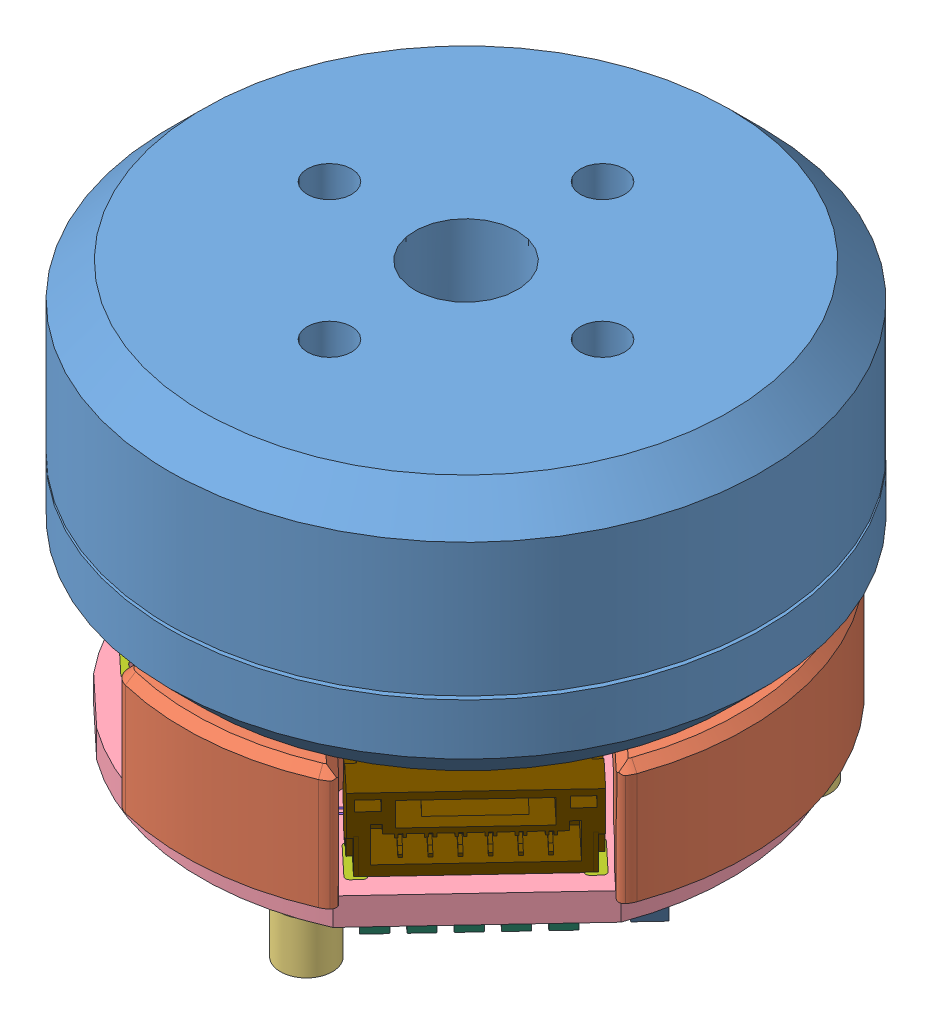
SolidWorks assembly 2804一体化电机, configuration 默认. Lengths in mm.
Overall size (43.63 26.6 43.64).
107 component instances, 59 part files, 14 mates.
Components (placement in the parent):
- 2804电机-typeC-1: 2804电机-typeC [默认] at (5.0798 -9.5399 34.8) size (34.8 18.5 34.8)
- 2804-驱动板支撑-1: 2804-驱动板支撑 [默认] at (5.0798 -16.5399 34.8) x (0.684211 0 -0.729285) z (0.729285 0 0.684211) size (31.01 7.3 30.73)
- 零件62^2804一体化电机-1: 零件62^2804一体化电机 [默认] at (146.4293 -18.1399 30.2926) x (-0.729285 0 -0.684211) z (0 -1 0) size (27.3 24.05 3) (virtual)
- 45度支架-1: 45度支架 [默认] at (-8.6044 -19.1399 49.3857) x (0.48381 -0.707107 -0.515682) z (-0.48381 -0.707107 0.515682) size (37.34 60 48.63) (hidden)
- 卧式支架-1: 卧式支架 [默认] at (19.6851 -22.6399 38.2185) x (0 1 0) z (0.973684 0 0.227902) size (33.58 34 57.06) (hidden)
- NANO SFOC S28PR-I2C-AS56001-NANO SFOC S28PR-I2C-AS5600-1: NANO SFOC S28PR-I2C-AS56001-NANO SFOC S28PR-I2C-AS5600 [默认] at (5.0801 -18.1399 34.8) x (-0.729285 0 -0.684211) z (0 -1 0) size (28.6 30.74 7.59)
  - NANO SFOC S28PR-I2C-AS56001-NANO SFOC S28PR-I2C-AS5600.step-1: NANO SFOC S28PR-I2C-AS56001-NANO SFOC S28PR-I2C-AS5600.step [默认] at origin size (28.6 30.74 10.35)
    - Board_Geoms_1e90.step-1: Board_Geoms_1e90.step [默认] at origin size (28.6 30.74 1.66)
      - Pcb_1e90.step-1: Pcb_1e90.step [默认] at (-99.9998 99.9998 0) size (28.6 30.74 1.6)
      - topPads_1e90.step-1: topPads_1e90.step [默认] at (-99.9998 99.9998 0.02) size (26.72 28.47 0.01)
      - topTracks_1e90.step-1: topTracks_1e90.step [默认] at (-99.9998 99.9998 0.01) size (27.11 27.21 0.04)
      - botPads_1e90.step-1: botPads_1e90.step [默认] at (-99.9998 99.9998 -1.62) size (26.48 28.47 0.01)
      - botTracks_1e90.step-1: botTracks_1e90.step [默认] at (-99.9998 99.9998 -1.61) size (25.33 20.82 0.01)
      - botZones_1e90.step-1: botZones_1e90.step [默认] at (-99.9998 99.9998 -1.61) size (4.83 3.95 0.02)
    - Step_Models_1e90.step-1: Step_Models_1e90.step [默认] at origin size (25.95 29.8 10.35)
      - Top_1e90.step-1: Top_1e90.step [默认] at origin size (25.86 24.98 1.75)
        - U3_PWP059_00006012a0b9.step-1: U3_PWP059_00006012a0b9.step [默认] at (-0.0198 -8.0402 0) x (0 1 0) z (1 0 0) size (6.4 1.2 9.7)
          - PWP28.step-1: PWP28.step [默认] at origin size (1 0.75 0.24)
          - PWP029.step-1: PWP029.step [默认] at origin size (1 0.75 0.24)
          - PWP030.step-1: PWP030.step [默认] at origin size (1 0.75 0.24)
          - PWP031.step-1: PWP031.step [默认] at origin size (1 0.75 0.24)
          - PWP032.step-1: PWP032.step [默认] at origin size (1 0.75 0.24)
          - PWP033.step-1: PWP033.step [默认] at origin size (1 0.75 0.24)
          - PWP034.step-1: PWP034.step [默认] at origin size (1 0.75 0.24)
          - PWP035.step-1: PWP035.step [默认] at origin size (1 0.75 0.24)
          - PWP036.step-1: PWP036.step [默认] at origin size (1 0.75 0.24)
          - PWP037.step-1: PWP037.step [默认] at origin size (1 0.75 0.24)
          - PWP038.step-1: PWP038.step [默认] at origin size (1 0.75 0.24)
          - PWP039.step-1: PWP039.step [默认] at origin size (1 0.75 0.24)
          - PWP040.step-1: PWP040.step [默认] at origin size (1 0.75 0.24)
          - PWP041.step-1: PWP041.step [默认] at origin size (1 0.75 0.24)
          - PWP042.step-1: PWP042.step [默认] at origin size (1 0.75 0.24)
          - PWP043.step-1: PWP043.step [默认] at origin size (1 0.75 0.24)
          - PWP044.step-1: PWP044.step [默认] at origin size (1 0.75 0.24)
          - PWP045.step-1: PWP045.step [默认] at origin size (1 0.75 0.24)
          - PWP046.step-1: PWP046.step [默认] at origin size (1 0.75 0.24)
          - PWP047.step-1: PWP047.step [默认] at origin size (1 0.75 0.24)
          - PWP048.step-1: PWP048.step [默认] at origin size (1 0.75 0.24)
          - PWP049.step-1: PWP049.step [默认] at origin size (1 0.75 0.24)
          - PWP050.step-1: PWP050.step [默认] at origin size (1 0.75 0.24)
          - PWP051.step-1: PWP051.step [默认] at origin size (1 0.75 0.24)
          - PWP052.step-1: PWP052.step [默认] at origin size (1 0.75 0.24)
          - PWP053.step-1: PWP053.step [默认] at origin size (1 0.75 0.24)
          - PWP054.step-1: PWP054.step [默认] at origin size (1 0.75 0.24)
          - PWP055.step-1: PWP055.step [默认] at origin size (1 0.75 0.24)
          - PWP056.step-1: PWP056.step [默认] at origin size (0.55 0.05 0.55)
          - PWP057.step-1: PWP057.step [默认] at origin size (4.4 1.06 9.7)
          - PWP058.step-1: PWP058.step [默认] at origin size (2.75 0.25 5.23)
        - C1_C_0603_1608Metric_00006005682b.step-1: C1_C_0603_1608Metric_00006005682b.step [默认] at (-5.0998 -1.0402 0) x (0 -1 0) z (0 0 1) size (1.6 0.8 0.8)
        - C1_C_0603_1608Metric_00006005682b.step-2: C1_C_0603_1608Metric_00006005682b.step [默认] at (-5.9698 -10.4127 0) x (0 -1 0) z (0 0 1) size (1.6 0.8 0.8)
        - C1_C_0603_1608Metric_00006005682b.step-3: C1_C_0603_1608Metric_00006005682b.step [默认] at (6.0402 -10.6702 0) x (0 1 0) z (0 0 1) size (1.6 0.8 0.8)
        - C1_C_0603_1608Metric_00006005682b.step-4: C1_C_0603_1608Metric_00006005682b.step [默认] at (-5.8223 -12.6402 0) x (-1 0 0) z (0 0 1) size (1.6 0.8 0.8)
        - C1_C_0603_1608Metric_00006005682b.step-5: C1_C_0603_1608Metric_00006005682b.step [默认] at (-7.4598 -10.4002 0) x (0 1 0) z (0 0 1) size (1.6 0.8 0.8)
        - C1_C_0603_1608Metric_00006005682b.step-6: C1_C_0603_1608Metric_00006005682b.step [默认] at (7.5302 -9.1502 0) x (0 -1 0) z (0 0 1) size (1.6 0.8 0.8)
        - D1_LED_0603_1608Metric_0000600568f0.step-1: D1_LED_0603_1608Metric_0000600568f0.step [默认] at (-7.4698 -7.4102 0) x (0 1 0) z (0 0 1) size (1.6 0.8 1.1)
        - R3_R_0603_1608Metric_0000600569a0.step-1: R3_R_0603_1608Metric_0000600569a0.step [默认] at (-8.9598 -7.4102 0) x (0 1 0) z (0 0 1) size (1.6 0.8 0.45)
        - R3_R_0603_1608Metric_0000600569a0.step-2: R3_R_0603_1608Metric_0000600569a0.step [默认] at (9.0402 -4.6902 0) x (0 -1 0) z (0 0 1) size (1.6 0.8 0.45)
        - R3_R_0603_1608Metric_0000600569a0.step-3: R3_R_0603_1608Metric_0000600569a0.step [默认] at (6.0402 -7.6827 0) x (0 -1 0) z (0 0 1) size (1.6 0.8 0.45)
        - C1_C_0603_1608Metric_00006005682b.step-7: C1_C_0603_1608Metric_00006005682b.step [默认] at (8.3002 -6.9202 0) size (1.6 0.8 0.8)
        - D2_D_0603_00006081285b.step-1: D2_D_0603_00006081285b.step [默认] at (7.5502 -4.6902 0) x (0 1 0) z (0 0 1) size (1.6 0.87 0.66)
        - R3_R_0603_1608Metric_0000600569a0.step-4: R3_R_0603_1608Metric_0000600569a0.step [默认] at (-6.6498 9.6598 0) x (-1 0 0) z (0 0 1) size (1.6 0.8 0.45)
        - R3_R_0603_1608Metric_0000600569a0.step-5: R3_R_0603_1608Metric_0000600569a0.step [默认] at (-6.6373 11.1498 0) size (1.6 0.8 0.45)
        - C1_C_0603_1608Metric_00006005682b.step-8: C1_C_0603_1608Metric_00006005682b.step [默认] at (-7.3998 7.4373 0) x (0 -1 0) z (0 0 1) size (1.6 0.8 0.8)
        - C1_C_0603_1608Metric_00006005682b.step-9: C1_C_0603_1608Metric_00006005682b.step [默认] at (-5.8998 7.4198 0) x (0 -1 0) z (0 0 1) size (1.6 0.8 0.8)
        - U4_SOIC_8_39x49mm_P127mm_00006143c6c9.step-1: U4_SOIC_8_39x49mm_P127mm_00006143c6c9.step [默认] at (-1.3798 8.8698 0) x (-1 0 0) z (0 0 1) size (6 4.9 1.75)
        - C1_C_0603_1608Metric_00006005682b.step-10: C1_C_0603_1608Metric_00006005682b.step [默认] at (-8.2098 1.4423 0) x (-1 0 0) z (0 0 1) size (1.6 0.8 0.8)
        - C1_C_0603_1608Metric_00006005682b.step-11: C1_C_0603_1608Metric_00006005682b.step [默认] at (-8.9598 -4.4102 0) x (0 1 0) z (0 0 1) size (1.6 0.8 0.8)
        - C1_C_0603_1608Metric_00006005682b.step-12: C1_C_0603_1608Metric_00006005682b.step [默认] at (-8.2073 2.9298 0) x (-1 0 0) z (0 0 1) size (1.6 0.8 0.8)
        - C1_C_0603_1608Metric_00006005682b.step-13: C1_C_0603_1608Metric_00006005682b.step [默认] at (-9.6498 9.0998 0) x (-1 0 0) z (0 0 1) size (1.6 0.8 0.8)
        - C1_C_0603_1608Metric_00006005682b.step-14: C1_C_0603_1608Metric_00006005682b.step [默认] at (-11.8073 5.3798 0) x (-1 0 0) z (0 0 1) size (1.6 0.8 0.8)
        - C19_C_1206_3216Metric_0000619d7bf4.step-1: C19_C_1206_3216Metric_0000619d7bf4.step [默认] at (-10.4298 7.2398 0) x (-1 0 0) z (0 0 1) size (3.2 1.6 1.6)
        - C19_C_1206_3216Metric_0000619d7bf4.step-2: C19_C_1206_3216Metric_0000619d7bf4.step [默认] at (-3.4598 4.8098 0) size (3.2 1.6 1.6)
        - D4_D_SOD_323_0000619d7c30.step-1: D4_D_SOD_323_0000619d7c30.step [默认] at (-4.8798 2.0698 0) x (0 1 0) z (0 0 1) size (2.5 1.25 1.1)
        - D4_D_SOD_323_0000619d7c30.step-2: D4_D_SOD_323_0000619d7c30.step [默认] at (-2.9398 2.0798 0) x (0 1 0) z (0 0 1) size (2.5 1.25 1.1)
        - L1_L_1206_3216Metric_0000619d7c59.step-1: L1_L_1206_3216Metric_0000619d7c59.step [默认] at (-8.0398 4.8198 0) size (3.2 1.6 1.6)
        - R3_R_0603_1608Metric_0000600569a0.step-6: R3_R_0603_1608Metric_0000600569a0.step [默认] at (-7.4698 -4.4002 0) x (0 1 0) z (0 0 1) size (1.6 0.8 0.45)
        - R3_R_0603_1608Metric_0000600569a0.step-7: R3_R_0603_1608Metric_0000600569a0.step [默认] at (-5.9698 -7.4102 0) x (0 -1 0) z (0 0 1) size (1.6 0.8 0.45)
        - R3_R_0603_1608Metric_0000600569a0.step-8: R3_R_0603_1608Metric_0000600569a0.step [默认] at (-5.9998 -4.4102 0) x (0 1 0) z (0 0 1) size (1.6 0.8 0.45)
        - U5_SOT_23_6_0000619d7cb3.step-1: U5_SOT_23_6_0000619d7cb3.step [默认] at (-7.7798 -1.1202 0) size (2.8 2.9 1.55)
        - U2_LQFP_48_7x7mm_P05mm_000061a3530d.step-1: U2_LQFP_48_7x7mm_P05mm_000061a3530d.step [默认] at (8.3102 2.0873 0) size (9 9 1.5)
        - C2_C_0805_2012Metric_40c0a07bab88.step-1: C2_C_0805_2012Metric_40c0a07bab88.step [默认] at (-12.0498 -0.2802 0) size (2 1.25 1.25)
        - C2_C_0805_2012Metric_40c0a07bab88.step-2: C2_C_0805_2012Metric_40c0a07bab88.step [默认] at (-12.0498 -4.2002 0) size (2 1.25 1.25)
        - C1_C_0603_1608Metric_00006005682b.step-15: C1_C_0603_1608Metric_00006005682b.step [默认] at (3.0802 6.7398 0) x (0 -1 0) z (0 0 1) size (1.6 0.8 0.8)
        - C1_C_0603_1608Metric_00006005682b.step-16: C1_C_0603_1608Metric_00006005682b.step [默认] at (10.6102 8.7548 0) x (0 -1 0) z (0 0 1) size (1.6 0.8 0.8)
        - C1_C_0603_1608Metric_00006005682b.step-17: C1_C_0603_1608Metric_00006005682b.step [默认] at (8.4502 10.6798 0) x (0 -1 0) z (0 0 1) size (1.6 0.8 0.8)
        - R3_R_0603_1608Metric_0000600569a0.step-9: R3_R_0603_1608Metric_0000600569a0.step [默认] at (-3.6298 -1.0302 0) x (0 1 0) z (0 0 1) size (1.6 0.8 0.45)
        - C2_C_0805_2012Metric_40c0a07bab88.step-3: C2_C_0805_2012Metric_40c0a07bab88.step [默认] at (-12.0498 3.6398 0) size (2 1.25 1.25)
        - C1_C_0603_1608Metric_00006005682b.step-18: C1_C_0603_1608Metric_00006005682b.step [默认] at (3.0352 -2.3302 0) size (1.6 0.8 0.8)
        - C1_C_0603_1608Metric_00006005682b.step-19: C1_C_0603_1608Metric_00006005682b.step [默认] at (11.2702 -3.9402 0) size (1.6 0.8 0.8)
        - R3_R_0603_1608Metric_0000600569a0.step-10: R3_R_0603_1608Metric_0000600569a0.step [默认] at (8.3602 7.9898 0) size (1.6 0.8 0.45)
        - C2_C_0805_2012Metric_40c0a07bab88.step-4: C2_C_0805_2012Metric_40c0a07bab88.step [默认] at (-12.0498 -2.2402 0) size (2 1.25 1.25)
        - C1_C_0603_1608Metric_00006005682b.step-20: C1_C_0603_1608Metric_00006005682b.step [默认] at (0.0752 -2.3102 0) x (-1 0 0) z (0 0 1) size (1.6 0.8 0.8)
        - R3_R_0603_1608Metric_0000600569a0.step-11: R3_R_0603_1608Metric_0000600569a0.step [默认] at (6.0602 -4.6902 0) x (0 -1 0) z (0 0 1) size (1.6 0.8 0.45)
        - C1_C_0603_1608Metric_00006005682b.step-21: C1_C_0603_1608Metric_00006005682b.step [默认] at (3.1202 9.7198 0) x (0 -1 0) z (0 0 1) size (1.6 0.8 0.8)
        - C2_C_0805_2012Metric_40c0a07bab88.step-5: C2_C_0805_2012Metric_40c0a07bab88.step [默认] at (-12.0498 1.6798 0) size (2 1.25 1.25)
        - R3_R_0603_1608Metric_0000600569a0.step-12: R3_R_0603_1608Metric_0000600569a0.step [默认] at (-2.1398 -1.0202 0) x (0 -1 0) z (0 0 1) size (1.6 0.8 0.45)
        - R3_R_0603_1608Metric_0000600569a0.step-13: R3_R_0603_1608Metric_0000600569a0.step [默认] at (9.0202 -9.1602 0) x (0 1 0) z (0 0 1) size (1.6 0.8 0.45)
        - R3_R_0603_1608Metric_0000600569a0.step-14: R3_R_0603_1608Metric_0000600569a0.step [默认] at (5.3502 7.9898 0) size (1.6 0.8 0.45)
        - VR1_SOT_23_ecdd3c14c820.step-1: VR1_SOT_23_ecdd3c14c820.step [默认] at (5.8002 10.4398 0) x (-1 0 0) z (0 0 1) size (2.5 3 1.2)
        - C1_C_0603_1608Metric_00006005682b.step-22: C1_C_0603_1608Metric_00006005682b.step [默认] at (0.8402 5.3998 0) x (-1 0 0) z (0 0 1) size (1.6 0.8 0.8)
      - Bot_1e90.step-1: Bot_1e90.step [默认] at origin size (25.86 29.8 10.1)
        - J1_PinSocket_1x03_P254mm_Vertical_00006005697e.step-1: J1_PinSocket_1x03_P254mm_Vertical_00006005697e.step [默认] at (2.5402 -13.4002 -1.6) x (0 1 0) z (0 0 -1) size (2.54 7.62 10.1) (hidden)
        - J4_SM06B-SRSS_00006030bad4[2].step-1: J4_SM06B-SRSS_00006030bad4[2].step [默认] at (9.0002 -0.0002 -1.35) x (0 -1 0) z (1 0 0) size (8 2.96 4.95)
        - U4_SOIC_8_39x49mm_P127mm_00006143c6c9.step-1: U4_SOIC_8_39x49mm_P127mm_00006143c6c9.step [默认] at (0.0002 -0.0002 -1.6) x (1 0 0) z (0 0 -1) size (6 4.9 1.75)
        - J3_JST_SM06B_GHS_TB_00006196b6b3.step-1: J3_JST_SM06B_GHS_TB_00006196b6b3.step [默认] at (-10.4929 -0.0002 -1.6) x (0 1 0) z (0 0 -1) size (10.75 4.95 4.25)
        - SW2_Selector Switch - MSK1103_cc7121352cae.step-1: SW2_Selector Switch - MSK1103_cc7121352cae.step [默认] at (2.7947 14.0863 -1.6) x (0.848048 -0.529919 0) z (0.529919 0.848048 0) size (7.98 2.01 6.19)
  - 零件111^NANO SFOC S28PR-I2C-AS56001-NANO SFOC S28PR-I2C-AS5600-1: 零件111^NANO SFOC S28PR-I2C-AS56001-NANO SFOC S28PR-I2C-AS5600 [默认] at (0.7088 1.5136 0) x (1 0 0) z (0 -1 0) size (3 0.8 4.6) (virtual)
Mates (geometry in assembly coordinates):
- 重合1: coincident anti-aligned: plane of 2804电机-typeC-1 through (5.0798 -9.5399 34.8) normal (0 -1 0); plane of 2804-驱动板支撑-1 through (5.0798 -9.5399 34.8) normal (0 1 0)
- 同心1: concentric aligned: cylinder of 2804电机-typeC-1 through (-4.4202 -4.5399 34.8) axis (0 -1 0) radius 1.3; cylinder of 2804-驱动板支撑-1 through (-4.4202 9.4601 34.8) axis (0 -1 0) radius 1.625
- 同心2: concentric aligned: cylinder of 2804电机-typeC-1 through (5.0798 -4.5399 34.8) axis (0 -1 0) radius 17.4; cylinder of 2804-驱动板支撑-1 through (5.0798 -9.5399 34.8) axis (0 -1 0) radius 16.5
- 重合3: coincident anti-aligned: plane of 铜柱M2x3-1 through (9.1324 -21.1399 48.2006) normal (0 -1 0); plane of 复件 零件25^2804一体化电机-1 through (5.0798 -21.1399 34.8) normal (0 1 0)
- 同心5: concentric anti-aligned: cylinder of 2804电机-typeC-1 through (5.0798 5.4601 34.8) axis (0 -1 0) radius 17.4; cylinder of 复件 零件25^2804一体化电机-1 through (5.0798 -61.1399 34.8) axis (0 1 0) radius 10
- 同心6: concentric aligned: cylinder of 铜柱M2x3-1 through (14.6588 -21.1399 24.59) axis (0 1 0) radius 1.1; cylinder of 复件 零件25^2804一体化电机-1 through (14.6588 -41.6148 24.59) axis (0 1 0) radius 2.5
- 重合4: coincident anti-aligned: plane of 铜柱M2x3-1 through (-8.5518 -21.1399 31.6094) normal (0 -1 0); plane of 卧式支架-1 through (-19.2419 -21.1399 46.5667) normal (0 1 0)
- 同心7: concentric anti-aligned: cylinder of 2804电机-typeC-1 through (5.0798 5.4601 34.8) axis (0 -1 0) radius 17.4; cylinder of 卧式支架-1 through (5.0798 -37.6399 34.8) axis (0 1 0) radius 7.5
- 同心8: concentric aligned: cylinder of 铜柱M2x3-1 through (9.1324 -21.1399 48.2006) axis (0 1 0) radius 1.1; cylinder of 卧式支架-1 through (9.1324 -37.6399 48.2006) axis (0 1 0) radius 1.1
- 重合5: coincident anti-aligned: plane of 2804-驱动板支撑-1 through (5.0798 -16.5399 34.8) normal (0 -1 0); plane of NANO SFOC S28PR-I2C-AS56001-NANO SFOC S28PR-I2C-AS5600-1/NANO SFOC S28PR-I2C-AS56001-NANO SFOC S28PR-I2C-AS5600.step-1/Board_Geoms_1e90.step-1/Pcb_1e90.step-1 through (5.08 -16.5399 34.8) normal (0 1 0)
- 同心9: concentric aligned: cylinder of 2804-驱动板支撑-1 through (5.0798 -9.5399 34.8) axis (0 -1 0) radius 16.5; cylinder of NANO SFOC S28PR-I2C-AS56001-NANO SFOC S28PR-I2C-AS5600-1/NANO SFOC S28PR-I2C-AS56001-NANO SFOC S28PR-I2C-AS5600.step-1/Board_Geoms_1e90.step-1/Pcb_1e90.step-1 through (5.0798 -18.1399 34.8) axis (0 -1 0) radius 15.4963
- 同心10: concentric anti-aligned: cylinder of 铜柱M2x3-1 through (14.6588 -21.1399 24.59) axis (0 1 0) radius 1.525; cylinder of NANO SFOC S28PR-I2C-AS56001-NANO SFOC S28PR-I2C-AS5600-1/NANO SFOC S28PR-I2C-AS56001-NANO SFOC S28PR-I2C-AS5600.step-1/Board_Geoms_1e90.step-1/Pcb_1e90.step-1 through (14.6588 -18.1399 24.59) axis (0 -1 0) radius 1.1
- 同心11: concentric anti-aligned: cylinder of 2804-驱动板支撑-1 through (14.6588 -17.5399 24.59) axis (0 1 0) radius 0.875; cylinder of NANO SFOC S28PR-I2C-AS56001-NANO SFOC S28PR-I2C-AS5600-1/NANO SFOC S28PR-I2C-AS56001-NANO SFOC S28PR-I2C-AS5600.step-1/Board_Geoms_1e90.step-1/Pcb_1e90.step-1 through (14.6588 -18.1399 24.59) axis (0 -1 0) radius 1.1
- 重合6: coincident anti-aligned: plane of 铜柱M2x3-1 through (14.6588 -18.1399 24.59) normal (0 1 0); plane of NANO SFOC S28PR-I2C-AS56001-NANO SFOC S28PR-I2C-AS5600-1/NANO SFOC S28PR-I2C-AS56001-NANO SFOC S28PR-I2C-AS5600.step-1/Board_Geoms_1e90.step-1/Pcb_1e90.step-1 through (5.08 -18.1399 34.8) normal (0 -1 0)
